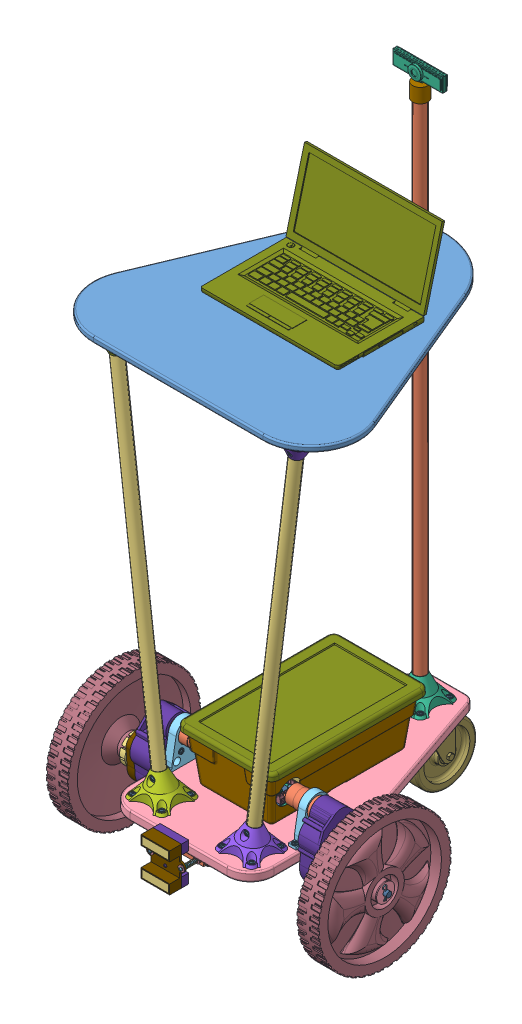
SolidWorks assembly Layla, configuration Default. Lengths in mm.
Overall size (589.28 1385.2 660.47).
388 component instances, 98 part files, 227 mates.
Components (placement in the parent):
- Layla_Top-1: Layla_Top [Default] at (-0.0562 830.9031 1403.6246) x (1 0 0.000267) z (-0.000267 0 1) size (558.8 12.7 558.8)
- Conduit_Back-1: Conduit_Back [Default] at (0.0274 577.85 997.2192) x (0.999959 0 0.009056) z (0 -1 0) size (24.13 24.13 1117.6)
- Conduit_Front-1: Conduit_Front [Default] at (144.1046 424.9766 1445.553) x (-0.000009 0 1) z (-0.121869 -0.992546 -0.000001) size (24.13 24.13 812.8)
- Conduit_Front-2: Conduit_Front [Default] at (-144.1046 424.9766 1445.553) x (0.000009 0 1) z (0.121869 -0.992546 -0.000001) size (24.13 24.13 812.8)
- Layla_Bottom-1: Layla_Bottom [Default] at (0.0001 0 1480.0562) x (1 0 0.000005) z (-0.000005 0 1) size (301.62 19.05 565.15)
- motor_bracket-1: motor_bracket [Default] at (128.32 -6.1562 1357.0318) x (0 1 0) z (1 0 0.000005) size (80.83 90 16)
- motor_bracket-2: motor_bracket [Default] at (-128.32 -6.1562 1357.0318) x (0 1 0) z (-1 0 0.000005) size (80.83 90 16)
- frame_bracket_volcano_back-1: frame_bracket_volcano_back [Default] at (0.0274 830.9031 997.2192) x (-0.00113 0 -0.999999) z (0 -1 0) size (90.91 90.9 52.13)
- frame_bracket_volcano_back-2: frame_bracket_volcano_back [Default] at (-0.0308 19.05 997.3051) x (-0.001001 0 -0.999999) z (0 1 0) size (90.91 90.9 52.13)
- frame_bracket_volcano_right-1: frame_bracket_volcano_right [Default] at (-94.2631 19.05 1445.5525) x (0.000009 0 1) z (0 1 0) size (90.91 90.9 53.32)
- frame_bracket_volcano_left-1: frame_bracket_volcano_left [Default] at (94.2631 19.05 1445.5525) x (-0.000009 0 1) z (0 -1 0) size (90.91 90.9 53.32)
- frame_bracket_volcano_right-2: frame_bracket_volcano_right [Default] at (-193.9461 830.9031 1445.5534) x (0.000009 0 1) z (0 -1 0) size (90.91 90.9 53.32)
- frame_bracket_volcano_left-2: frame_bracket_volcano_left [Default] at (193.9461 830.9031 1445.5534) x (-0.000009 0 1) z (0 1 0) size (90.91 90.9 53.32)
- Camera_Bracket-1: Camera_Bracket [Default] at (0.0274 1112.52 997.2192) x (0.105259 0 -0.994445) z (0.994445 0 0.105259) size (31.75 29.97 31.75)
- Axle_7_16-2: Axle_7_16 [Default] at (0.0008 -8.865 1357.1611) x (0.000005 -0.039071 -0.999236) z (1 0 0.000005) size (11.11 11.11 589.28)
- axle_bracket_7_16-1: axle_bracket_7_16 [Default] at (82.3318 -8.885 1357.1616) x (-0.000005 0 1) z (1 0 0.000005) size (44.81 15.79 16.5)
- axle_bracket_7_16-2: axle_bracket_7_16 [Default] at (-82.3303 -8.885 1357.1607) x (-0.000005 0 1) z (1 0 0.000005) size (44.81 15.79 16.5)
- Caster Part-1: Caster Part [Default] at (176.8474 -193.4184 944.9392) x (-1 0 -0.000005) z (0.000005 0 -1) size (73 156.46 148.87)
- 11in_Mower_Wheel-5: 11in_Mower_Wheel [Default] at (285.3317 -8.865 1357.1626) x (-0.000004 0.731602 0.681732) z (-1 0 -0.000005) size (279.4 279.4 57.46)
- 11in_Mower_Wheel-6: 11in_Mower_Wheel [Default] at (-285.3301 -8.865 1357.1596) x (-0.000005 0.394974 0.918692) z (1 0 0.000005) size (279.4 279.4 57.46)
- Screw_8_(0.75'')-1: Screw_8_(0.75'') [Default] at (-22.2101 9.652 1035.0706) x (-1 0 0) z (0 0 1) size (10.85 21.85 10.85)
- Screw_8_(0.75'')-2: Screw_8_(0.75'') [Default] at (22.2149 9.652 1035.0709) x (-1 0 0) z (0 0 1) size (10.85 21.85 10.85)
- Screw_8_(0.75'')-3: Screw_8_(0.75'') [Default] at (22.2153 9.652 958.9459) x (-1 0 0) z (0 0 1) size (10.85 21.85 10.85)
- Screw_8_(0.75'')-4: Screw_8_(0.75'') [Default] at (-22.2097 9.652 958.9456) x (-1 0 0) z (0 0 1) size (10.85 21.85 10.85)
- Screw_8_(0.75'')-5: Screw_8_(0.75'') [Default] at (82.3319 7.5213 1341.0054) x (-1 0 0) z (0 0 1) size (10.85 21.85 10.85)
- Screw_8_(0.75'')-7: Screw_8_(0.75'') [Default] at (-82.3303 7.5213 1373.3169) x (-1 0 0) z (0 0 1) size (10.85 21.85 10.85)
- Screw_8_(0.75'')-9: Screw_8_(0.75'') [Default] at (124.3148 10.35 1475.6049) x (-1 0 0) z (0 0 -1) size (10.85 21.85 10.85)
- Screw_8_(0.75'')-10: Screw_8_(0.75'') [Default] at (124.3154 10.35 1415.5008) x (-1 0 0) z (0 0 -1) size (10.85 21.85 10.85)
- Screw_8_(0.75'')-11: Screw_8_(0.75'') [Default] at (64.2113 10.35 1415.5002) x (-1 0 0) z (0 0 -1) size (10.85 21.85 10.85)
- Screw_8_(0.75'')-12: Screw_8_(0.75'') [Default] at (64.2107 10.35 1475.6043) x (-1 0 0) z (0 0 -1) size (10.85 21.85 10.85)
- Screw_8_(0.75'')-13: Screw_8_(0.75'') [Default] at (-64.2107 10.35 1475.6043) x (-1 0 0) z (0 0 -1) size (10.85 21.85 10.85)
- Screw_8_(0.75'')-14: Screw_8_(0.75'') [Default] at (-124.3148 10.35 1475.6049) x (-1 0 0) z (0 0 -1) size (10.85 21.85 10.85)
- Screw_8_(0.75'')-15: Screw_8_(0.75'') [Default] at (-124.3154 10.35 1415.5008) x (-1 0 0) z (0 0 -1) size (10.85 21.85 10.85)
- Screw_8_(0.75'')-17: Screw_8_(0.75'') [Default] at (-64.2113 10.35 1415.5002) x (-1 0 0) z (0 0 -1) size (10.85 21.85 10.85)
- Screw_8_(0.75'')-18: Screw_8_(0.75'') [Default] at (-136.3198 11.314 1395.7818) x (-1 0 0) z (0 0 -1) size (10.85 21.85 10.85)
- Screw_8_(0.75'')-19: Screw_8_(0.75'') [Default] at (-136.3202 11.314 1318.2818) x (-1 0 0) z (0 0 -1) size (10.85 21.85 10.85)
- Screw_8_(0.75'')-20: Screw_8_(0.75'') [Default] at (136.3198 11.314 1395.7818) x (-1 0 0) z (0 0 -1) size (10.85 21.85 10.85)
- Screw_8_(0.75'')-21: Screw_8_(0.75'') [Default] at (136.3202 11.314 1318.2818) x (-1 0 0) z (0 0 -1) size (10.85 21.85 10.85)
- Screw_8_(0.75'')-22: Screw_8_(0.75'') [Default] at (30.0513 10.35 1027.3271) x (-1 0 0) z (0 0 -1) size (10.85 21.85 10.85)
- Screw_8_(0.75'')-23: Screw_8_(0.75'') [Default] at (29.9912 10.35 967.223) x (-1 0 0) z (0 0 -1) size (10.85 21.85 10.85)
- Screw_8_(0.75'')-24: Screw_8_(0.75'') [Default] at (-30.1129 10.35 967.2832) x (-1 0 0) z (0 0 -1) size (10.85 21.85 10.85)
- Screw_8_(0.75'')-25: Screw_8_(0.75'') [Default] at (-30.0527 10.35 1027.3872) x (-1 0 0) z (0 0 -1) size (10.85 21.85 10.85)
- Screw_8_(0.75'')-28: Screw_8_(0.75'') [Default] at (-0.0319 56.55 996.1551) x (0 1 0) z (-0.999999 0 0.001001) size (10.85 21.85 10.85)
- Screw_8_(0.75'')-29: Screw_8_(0.75'') [Default] at (98.8331 56.2705 1446.7026) x (0 1 0) z (1 0 0.000009) size (10.85 21.85 10.85)
- Screw_8_(0.75'')-30: Screw_8_(0.75'') [Default] at (-98.8331 56.2705 1446.7026) x (0 1 0) z (1 0 -0.000009) size (10.85 21.85 10.85)
- Screw_8_(0.75'')-32: Screw_8_(0.75'') [Default] at (-189.376 793.6826 1446.7034) x (0 -1 0) z (-1 0 0.000009) size (10.85 21.85 10.85)
- Screw_8_(0.75'')-33: Screw_8_(0.75'') [Default] at (189.376 793.6826 1446.7034) x (0 1 0) z (1 0 0.000009) size (10.85 21.85 10.85)
- Screw_8_(0.75'')-34: Screw_8_(0.75'') [Default] at (0.0261 793.4031 996.0692) x (0 1 0) z (-0.999999 0 0.00113) size (10.85 21.85 10.85)
- Screw_8_(0.75'')-36: Screw_8_(0.75'') [Default] at (82.3317 7.5213 1373.3178) x (-1 0 0) z (0 0 1) size (10.85 21.85 10.85)
- Screw_8_(0.75'')-37: Screw_8_(0.75'') [Default] at (-82.3302 7.5213 1341.0045) x (-1 0 0) z (0 0 1) size (10.85 21.85 10.85)
- Screw_8_(0.75'')-38: Screw_8_(0.75'') [Default] at (-141.0199 47.7688 1371.1468) x (0.000005 0 1) z (0 1 0) size (10.85 21.85 10.85)
- Screw_8_(0.75'')-39: Screw_8_(0.75'') [Default] at (141.0201 47.7688 1342.9169) x (0.000005 0 -1) z (0 1 0) size (10.85 21.85 10.85)
- Screw_8_(0.5'')-1: Screw_8_(0.5'') [Default] at (223.9979 833.2531 1475.6057) x (-1 0 -0.000267) z (-0.000267 0 1) size (10.85 15.5 10.85)
- Screw_8_(0.5'')-2: Screw_8_(0.5'') [Default] at (163.8938 833.2531 1475.6052) x (-1 0 -0.000267) z (-0.000267 0 1) size (10.85 15.5 10.85)
- Screw_8_(0.5'')-3: Screw_8_(0.5'') [Default] at (163.8943 833.2531 1415.5011) x (-1 0 -0.000267) z (-0.000267 0 1) size (10.85 15.5 10.85)
- Screw_8_(0.5'')-4: Screw_8_(0.5'') [Default] at (223.9984 833.2531 1415.5017) x (-1 0 -0.000267) z (-0.000267 0 1) size (10.85 15.5 10.85)
- Screw_8_(0.5'')-6: Screw_8_(0.5'') [Default] at (-163.8938 833.2531 1475.6052) x (-1 0 -0.000267) z (-0.000267 0 1) size (10.85 15.5 10.85)
- Screw_8_(0.5'')-7: Screw_8_(0.5'') [Default] at (-223.9979 833.2531 1475.6057) x (-1 0 -0.000267) z (-0.000267 0 1) size (10.85 15.5 10.85)
- Screw_8_(0.5'')-8: Screw_8_(0.5'') [Default] at (-223.9984 833.2531 1415.5017) x (-1 0 -0.000267) z (-0.000267 0 1) size (10.85 15.5 10.85)
- Screw_8_(0.5'')-9: Screw_8_(0.5'') [Default] at (-163.8943 833.2531 1415.5011) x (-1 0 -0.000267) z (-0.000267 0 1) size (10.85 15.5 10.85)
- Screw_8_(0.5'')-10: Screw_8_(0.5'') [Default] at (30.1134 833.2531 1027.2373) x (-1 0 -0.000267) z (-0.000267 0 1) size (10.85 15.5 10.85)
- Screw_8_(0.5'')-11: Screw_8_(0.5'') [Default] at (-29.9907 833.2531 1027.3052) x (-1 0 -0.000267) z (-0.000267 0 1) size (10.85 15.5 10.85)
- Screw_8_(0.5'')-12: Screw_8_(0.5'') [Default] at (-30.0586 833.2531 967.2011) x (-1 0 -0.000267) z (-0.000267 0 1) size (10.85 15.5 10.85)
- Screw_8_(0.5'')-13: Screw_8_(0.5'') [Default] at (30.0455 833.2531 967.1332) x (-1 0 -0.000267) z (-0.000267 0 1) size (10.85 15.5 10.85)
- Laptop-2: Laptop [Default] at (-144.399 841.3074 1314.5854) size (290.36 165.51 224.16)
- Peg_Perego_Gearbox-1: Peg_Perego_Gearbox [Default] at (178.15 45.4709 1342.5236) x (0.000001 0.992561 -0.121745) z (-0.000005 0.121745 0.992561) size (150.54 143.03 103.18)
  - Peg_Perego_Gearbox_Bottom-1: Peg_Perego_Gearbox_Bottom [Default] at (-27.6979 -16.6053 10.3143) size (150.54 43.95 103.18)
  - Peg_Perego_Gearbox_Top-1: Peg_Perego_Gearbox_Top [Default] at (-40.5901 -16.6053 7.9144) x (-1 0 0) z (0 0 1) size (114.07 19.3 83.82)
  - Peg_Perego_Gearbox_Big_Gear-1: Peg_Perego_Gearbox_Big_Gear [Default] at (-55.7139 -16.6053 7.9144) x (-1 0 0) z (0 0 1) size (53.24 35.08 53.24)
  - Peg_Perego_Gearbox_Motor-1: Peg_Perego_Gearbox_Motor [Default] at (26.8065 84.3597 18.0362) x (0 0 1) z (1 0 0) size (37.46 84.84 37.46)
- Peg_Perego_Gearbox-8: Peg_Perego_Gearbox [Default] at (-178.1485 45.5433 1371.527) x (-0.000001 0.993157 0.116786) z (0.000005 0.116786 -0.993157) size (150.54 143.03 103.18)
  - Peg_Perego_Gearbox_Bottom-1: Peg_Perego_Gearbox_Bottom [Default] at (-27.6979 -16.6053 10.3143) size (150.54 43.95 103.18)
  - Peg_Perego_Gearbox_Top-1: Peg_Perego_Gearbox_Top [Default] at (-40.5901 -16.6053 7.9144) x (-1 0 0) z (0 0 1) size (114.07 19.3 83.82)
  - Peg_Perego_Gearbox_Big_Gear-1: Peg_Perego_Gearbox_Big_Gear [Default] at (-55.7139 -16.6053 7.9144) x (-1 0 0) z (0 0 1) size (53.24 35.08 53.24)
  - Peg_Perego_Gearbox_Motor-1: Peg_Perego_Gearbox_Motor [Default] at (26.8065 84.3597 18.0362) x (0 0 1) z (1 0 0) size (37.46 84.84 37.46)
- 11in_barbie_mower-1: 11in_barbie_mower [Default] at (241.7707 -8.865 1357.1624) x (0.000005 -0.121745 -0.992561) z (0.000001 0.992561 -0.121745) size (59.94 28.01 59.94)
- 11in_barbie_mower-3: 11in_barbie_mower [Default] at (-241.7691 -8.865 1357.1599) x (0.000001 -0.993157 -0.116786) z (-0.000005 -0.116786 0.993157) size (59.94 28.01 59.94)
- Washer_7_16-1: Washer_7_16 [Default] at (-287.3621 -8.865 1357.1596) x (-0.000004 0.592783 0.805362) z (1 0 0.000005) size (38.1 38.1 2.03)
- Washer_7_16-2: Washer_7_16 [Default] at (285.3317 -8.865 1357.1626) x (-0.000003 0.8256 0.564257) z (1 0 0.000005) size (38.1 38.1 2.03)
- Hair Pin Cotter Pin-1: Hair Pin Cotter Pin [Default] at (288.7988 -22.9437 1357.7131) x (0 0.999236 -0.039071) z (-0.000005 0.039071 0.999236) size (30.72 1.5 9.05)
- Hair Pin Cotter Pin-2: Hair Pin Cotter Pin [Default] at (-288.7972 -22.6511 1357.6986) x (0 0.999236 -0.039071) z (-0.000005 0.039071 0.999236) size (30.72 1.5 9.05)
- Genius_Webcam-1: Genius_Webcam [Default] at (0.0274 1163.8661 993.1679) size (105.03 41.22 29.03)
- Counterweight_Ingot-1: Counterweight_Ingot [Default] at (0.0022 0 1072.91) x (1 0 0.000005) z (0.000005 0 -1) size (106.83 31.75 49.05)
- Counterweight_Ingot_Screw-1: Counterweight_Ingot_Screw [Default] at (-28.5728 -32.25 1072.9098) x (-1 0 0) z (0 0 1) size (8 45 8)
- Counterweight_Ingot_Screw-2: Counterweight_Ingot_Screw [Default] at (28.5772 -32.25 1072.9101) x (-1 0 0) z (0 0 1) size (8 45 8)
- electronics_box-2: electronics_box [Default] at (6.4079 61.0311 1230.8661) x (-1 0 -0.000005) z (0.000005 0 -1) size (200.66 116.21 330.83)
  - sterilite_box-1: sterilite_box [Default] at (6.4065 -41.9824 -170.8478) size (195.22 114.3 325.39)
  - electronics_tray-1: electronics_tray [Default] at (67.0566 -75.9526 -72.8113) x (0 0 1) z (-1 0 0) size (203.2 36.13 152.4)
    - ibt2_assembly-1: ibt2_assembly [Default] at (25.1982 40.7289 22.1019) size (49.66 21.28 49.78)
      - IBT2_pcb-1: IBT2_pcb [Default] at (-57.2691 7.2367 24.7687) size (49.66 1.57 49.4)
      - header_male_2x4-1: header_male_2x4 [Default] at (4.8115 23.0826 24.5335) x (1 0 0) z (0 -1 0) size (10.16 5.08 10.92)
        - header_pin_base_2x4-1: header_pin_base_2x4 [Default] at (-49.9521 21.6346 11.7311) size (10.16 5.08 2.54)
        - header_pin-1: header_pin [Default] at (-56.3021 22.9046 6.0161) size (0.64 0.64 10.92)
        - header_pin-2: header_pin [Default] at (-56.3021 20.3646 6.0161) size (0.64 0.64 10.92)
        - header_pin-3: header_pin [Default] at (-53.7621 22.9046 6.0161) size (0.64 0.64 10.92)
        - header_pin-4: header_pin [Default] at (-53.7621 20.3646 6.0161) size (0.64 0.64 10.92)
        - header_pin-5: header_pin [Default] at (-51.2221 22.9046 6.0161) size (0.64 0.64 10.92)
        - header_pin-6: header_pin [Default] at (-51.2221 20.3646 6.0161) size (0.64 0.64 10.92)
        - header_pin-7: header_pin [Default] at (-48.6821 22.9046 6.0161) size (0.64 0.64 10.92)
        - header_pin-8: header_pin [Default] at (-48.6821 20.3646 6.0161) size (0.64 0.64 10.92)
      - AMP_screw-terminal_2POS_large-1: AMP_screw-terminal_2POS_large [Default] at (-57.2056 17.0115 0.4662) x (-1 0 0) z (0 0 -1) size (10.66 17 9)
      - AMP_screw-terminal_2POS_large-2: AMP_screw-terminal_2POS_large [Default] at (-47.0456 17.0115 0.4662) x (-1 0 0) z (0 0 -1) size (10.66 17 9)
      - cap_5mm_pitch-1: cap_5mm_pitch [Default] at (-68.3924 8.8115 4.7662) size (10.16 19.69 10.16)
      - d2pak-1: d2pak [Default] at (-63.2409 8.7779 25.6248) x (1 0 0) z (0 0.999978 0.006671) size (9.87 15.09 4.26)
      - d2pak-2: d2pak [Default] at (-52.336 8.7779 25.6248) x (1 0 0) z (0 0.999978 0.006671) size (9.87 15.09 4.26)
      - SOIC20 wide-1: SOIC20 wide [Default] at (-39.9304 8.5615 36.0347) x (1 0 0) z (0 1 0) size (13 10.17 2.01)
      - cap_0805-1: cap_0805 [Default] at (-38.0286 9.3449 27.3468) x (1 0 0) z (0 -1 0) size (2.03 1.32 0.56)
      - resistor_0805-1: resistor_0805 [Default] at (-48.3156 9.3449 41.6216) x (0 0 -1) z (0 -1 0) size (2.03 1.32 0.56)
      - resistor_0805-2: resistor_0805 [Default] at (-50.4517 9.3449 41.6216) x (0 0 -1) z (0 -1 0) size (2.03 1.32 0.56)
      - resistor_0805-3: resistor_0805 [Default] at (-52.5879 9.3449 41.6216) x (0 0 -1) z (0 -1 0) size (2.03 1.32 0.56)
      - resistor_0805-4: resistor_0805 [Default] at (-54.724 9.3449 41.6216) x (0 0 -1) z (0 -1 0) size (2.03 1.32 0.56)
      - resistor_0805-5: resistor_0805 [Default] at (-56.8602 9.3449 41.6216) x (0 0 -1) z (0 -1 0) size (2.03 1.32 0.56)
      - resistor_0805-6: resistor_0805 [Default] at (-58.9963 9.3449 41.6216) x (0 0 -1) z (0 -1 0) size (2.03 1.32 0.56)
      - resistor_0805-7: resistor_0805 [Default] at (-61.1324 9.3449 41.6216) x (0 0 -1) z (0 -1 0) size (2.03 1.32 0.56)
      - resistor_0805-8: resistor_0805 [Default] at (-63.2686 9.3449 41.6216) x (0 0 -1) z (0 -1 0) size (2.03 1.32 0.56)
    - ibt2_assembly-2: ibt2_assembly [Default] at (-89.34 40.7289 121.0422) x (-1 0 0) z (0 0 -1) size (49.66 21.28 49.78)
      - IBT2_pcb-1: IBT2_pcb [Default] at (-57.2691 7.2367 24.7687) size (49.66 1.57 49.4)
      - header_male_2x4-1: header_male_2x4 [Default] at (4.8115 23.0826 24.5335) x (1 0 0) z (0 -1 0) size (10.16 5.08 10.92)
        - header_pin_base_2x4-1: header_pin_base_2x4 [Default] at (-49.9521 21.6346 11.7311) size (10.16 5.08 2.54)
        - header_pin-1: header_pin [Default] at (-56.3021 22.9046 6.0161) size (0.64 0.64 10.92)
        - header_pin-2: header_pin [Default] at (-56.3021 20.3646 6.0161) size (0.64 0.64 10.92)
        - header_pin-3: header_pin [Default] at (-53.7621 22.9046 6.0161) size (0.64 0.64 10.92)
        - header_pin-4: header_pin [Default] at (-53.7621 20.3646 6.0161) size (0.64 0.64 10.92)
        - header_pin-5: header_pin [Default] at (-51.2221 22.9046 6.0161) size (0.64 0.64 10.92)
        - header_pin-6: header_pin [Default] at (-51.2221 20.3646 6.0161) size (0.64 0.64 10.92)
        - header_pin-7: header_pin [Default] at (-48.6821 22.9046 6.0161) size (0.64 0.64 10.92)
        - header_pin-8: header_pin [Default] at (-48.6821 20.3646 6.0161) size (0.64 0.64 10.92)
      - AMP_screw-terminal_2POS_large-1: AMP_screw-terminal_2POS_large [Default] at (-57.2056 17.0115 0.4662) x (-1 0 0) z (0 0 -1) size (10.66 17 9)
      - AMP_screw-terminal_2POS_large-2: AMP_screw-terminal_2POS_large [Default] at (-47.0456 17.0115 0.4662) x (-1 0 0) z (0 0 -1) size (10.66 17 9)
      - cap_5mm_pitch-1: cap_5mm_pitch [Default] at (-68.3924 8.8115 4.7662) size (10.16 19.69 10.16)
      - d2pak-1: d2pak [Default] at (-63.2409 8.7779 25.6248) x (1 0 0) z (0 0.999978 0.006671) size (9.87 15.09 4.26)
      - d2pak-2: d2pak [Default] at (-52.336 8.7779 25.6248) x (1 0 0) z (0 0.999978 0.006671) size (9.87 15.09 4.26)
      - SOIC20 wide-1: SOIC20 wide [Default] at (-39.9304 8.5615 36.0347) x (1 0 0) z (0 1 0) size (13 10.17 2.01)
      - cap_0805-1: cap_0805 [Default] at (-38.0286 9.3449 27.3468) x (1 0 0) z (0 -1 0) size (2.03 1.32 0.56)
      - resistor_0805-1: resistor_0805 [Default] at (-48.3156 9.3449 41.6216) x (0 0 -1) z (0 -1 0) size (2.03 1.32 0.56)
      - resistor_0805-2: resistor_0805 [Default] at (-50.4517 9.3449 41.6216) x (0 0 -1) z (0 -1 0) size (2.03 1.32 0.56)
      - resistor_0805-3: resistor_0805 [Default] at (-52.5879 9.3449 41.6216) x (0 0 -1) z (0 -1 0) size (2.03 1.32 0.56)
      - resistor_0805-4: resistor_0805 [Default] at (-54.724 9.3449 41.6216) x (0 0 -1) z (0 -1 0) size (2.03 1.32 0.56)
      - resistor_0805-5: resistor_0805 [Default] at (-56.8602 9.3449 41.6216) x (0 0 -1) z (0 -1 0) size (2.03 1.32 0.56)
      - resistor_0805-6: resistor_0805 [Default] at (-58.9963 9.3449 41.6216) x (0 0 -1) z (0 -1 0) size (2.03 1.32 0.56)
      - resistor_0805-7: resistor_0805 [Default] at (-61.1324 9.3449 41.6216) x (0 0 -1) z (0 -1 0) size (2.03 1.32 0.56)
      - resistor_0805-8: resistor_0805 [Default] at (-63.2686 9.3449 41.6216) x (0 0 -1) z (0 -1 0) size (2.03 1.32 0.56)
    - Arduino_mega-1: Arduino_mega [Default] at (5.4045 37.4555 130.5264) x (0 0 1) z (0 1 0) size (107.7 53.34 12.38)
      - Arduino_mega-1: Arduino_mega [Default] at (-98.4513 -6.297 10.51) size (101.6 53.34 1.59)
      - USB-jack-1: USB-jack [Default] at (-104.5473 25.6308 12.0975) size (16.46 12.14 10.79)
      - DC-jack-1: DC-jack [Default] at (-99.9245 -2.5632 12.0975) x (0 1 0) z (0 0 -1) size (8.79 13.59 10.72)
      - header_8-pin-1: header_8-pin [Default] at (-53.7727 -5.0778 12.0975) size (20.32 2.54 8.56)
      - header_8-pin-2: header_8-pin [Default] at (-30.6587 -5.0778 12.0975) size (20.32 2.54 8.56)
      - header_8-pin-3: header_8-pin [Default] at (-8.0781 -5.0778 12.0975) size (20.32 2.54 8.56)
      - header_8-pin-4: header_8-pin [Default] at (-35.7895 43.0044 12.0975) size (20.32 2.54 8.56)
      - header_8-pin-5: header_8-pin [Default] at (-13.1835 43.0044 12.0975) size (20.32 2.54 8.56)
      - header_10-pin-1: header_10-pin [Default] at (-58.0145 43.0044 12.0975) size (25.4 2.54 8.56)
      - header_36-pin-1: header_36-pin [Default] at (-0.5343 43.0298 12.0975) x (0 1 0) z (0 0 1) size (45.72 5.08 8.56)
    - arduino uno-1: arduino uno [Default] at (57.5276 49.6156 28.9001) x (-1 0 0) z (0 0 -1) size (53.34 15.25 74.97)
      - unoboard blue-1: unoboard blue [Default] at origin size (53.34 1.65 68.58)
      - 47uf CAP Dcase-1: 47uf CAP Dcase [Default] at (-9.4141 0 -18.4991) x (0 0 -1) z (1 0 0) size (6.6 5.81 8)
      - USB type b-1: USB type b [Default] at (-38.02 0.43 6.35) size (13.72 15.2 16.54)
        - USB SHELL-1: USB SHELL [Default] at origin size (13.72 15.2 16.54)
        - USB core-1: USB core [Default] at origin size (11.3 10.68 15.75)
        - usb top contact-1: usb top contact [Default] at (1.25 6.09 -0.38) size (1 9.67 13.76)
        - usb btm contact-1: usb btm contact [Default] at (1.25 4.41 -0.38) size (1 6.84 11.76)
        - usb btm contact-2: usb btm contact [Default] at (-1.25 4.41 -0.38) size (1 6.84 11.76)
        - usb top contact-2: usb top contact [Default] at (-1.25 6.09 -0.38) size (1 9.67 13.76)
      - power jack-1: power jack [Default] at (-7.675 0 1.905) size (11.2 15.2 15.9)
      - 47uf CAP Dcase-2: 47uf CAP Dcase [Default] at (-9.4141 0 -25.7132) x (0 0 -1) z (1 0 0) size (6.6 5.81 8)
      - crystal-1: crystal [Default] at (-26.162 0 -18.923) x (1 0 0) z (0 0 -1) size (4 5 11)
      - 2pin_header__02-1: 2pin_header__02 [Default] at (-46.23 0 -15.75) size (5 11.75 2.54)
      - nano - reg-1: nano - reg [Default] at (-17.399 0 -7.747) size (6.5 1.69 8.3)
      - led-1: led [Default] at (-34.29 0 -27.94) x (0 0 1) z (-1 0 0) size (4 0.86 1.35)
      - 2pin_header__02-2: 2pin_header__02 [Default] at (-30.43 0 -64.91) x (0 0 1) z (-1 0 0) size (5 11.75 2.54)
      - dip28-1: dip28 [Default] at (-16.383 1.5 -46.355) x (0 0 -1) z (1 0 0) size (35.48 7.37 10.1)
        - dip28-1: dip28 [Default] at origin size (35.48 2.8 10.1)
        - dip socket pin-1: dip socket pin [Default] at (16.51 2.8 -3.81) size (1.7 7.37 1.7)
        - dip socket pin-2: dip socket pin [Default] at (16.51 2.8 3.81) size (1.7 7.37 1.7)
        - dip socket pin-3: dip socket pin [Default] at (13.97 2.8 -3.81) size (1.7 7.37 1.7)
        - dip socket pin-4: dip socket pin [Default] at (13.97 2.8 3.81) size (1.7 7.37 1.7)
        - dip socket pin-5: dip socket pin [Default] at (11.43 2.8 -3.81) size (1.7 7.37 1.7)
        - dip socket pin-6: dip socket pin [Default] at (11.43 2.8 3.81) size (1.7 7.37 1.7)
        - dip socket pin-7: dip socket pin [Default] at (8.89 2.8 -3.81) size (1.7 7.37 1.7)
        - dip socket pin-8: dip socket pin [Default] at (8.89 2.8 3.81) size (1.7 7.37 1.7)
        - dip socket pin-9: dip socket pin [Default] at (6.35 2.8 -3.81) size (1.7 7.37 1.7)
        - dip socket pin-10: dip socket pin [Default] at (6.35 2.8 3.81) size (1.7 7.37 1.7)
        - dip socket pin-11: dip socket pin [Default] at (3.81 2.8 -3.81) size (1.7 7.37 1.7)
        - dip socket pin-12: dip socket pin [Default] at (3.81 2.8 3.81) size (1.7 7.37 1.7)
        - dip socket pin-13: dip socket pin [Default] at (1.27 2.8 -3.81) size (1.7 7.37 1.7)
        - dip socket pin-14: dip socket pin [Default] at (1.27 2.8 3.81) size (1.7 7.37 1.7)
        - dip socket pin-15: dip socket pin [Default] at (-1.27 2.8 -3.81) size (1.7 7.37 1.7)
        - dip socket pin-16: dip socket pin [Default] at (-1.27 2.8 3.81) size (1.7 7.37 1.7)
        - dip socket pin-17: dip socket pin [Default] at (-3.81 2.8 -3.81) size (1.7 7.37 1.7)
        - dip socket pin-18: dip socket pin [Default] at (-3.81 2.8 3.81) size (1.7 7.37 1.7)
        - dip socket pin-19: dip socket pin [Default] at (-6.35 2.8 -3.81) size (1.7 7.37 1.7)
        - dip socket pin-20: dip socket pin [Default] at (-6.35 2.8 3.81) size (1.7 7.37 1.7)
        - dip socket pin-21: dip socket pin [Default] at (-8.89 2.8 -3.81) size (1.7 7.37 1.7)
        - dip socket pin-22: dip socket pin [Default] at (-8.89 2.8 3.81) size (1.7 7.37 1.7)
        - dip socket pin-23: dip socket pin [Default] at (-11.43 2.8 -3.81) size (1.7 7.37 1.7)
        - dip socket pin-24: dip socket pin [Default] at (-11.43 2.8 3.81) size (1.7 7.37 1.7)
        - dip socket pin-25: dip socket pin [Default] at (-13.97 2.8 -3.81) size (1.7 7.37 1.7)
        - dip socket pin-26: dip socket pin [Default] at (-13.97 2.8 3.81) size (1.7 7.37 1.7)
        - dip socket pin-27: dip socket pin [Default] at (-16.51 2.8 -3.81) size (1.7 7.37 1.7)
        - dip socket pin-28: dip socket pin [Default] at (-16.51 2.8 3.81) size (1.7 7.37 1.7)
      - 2pin_header__02-3: 2pin_header__02 [Default] at (-27.89 0 -64.91) x (0 0 1) z (-1 0 0) size (5 11.75 2.54)
      - 2pin_header__02-4: 2pin_header__02 [Default] at (-25.35 0 -64.91) x (0 0 1) z (-1 0 0) size (5 11.75 2.54)
      - 2pin_header__02-5: 2pin_header__02 [Default] at (-46.23 0 -18.29) size (5 11.75 2.54)
      - 2pin_header__02-6: 2pin_header__02 [Default] at (-46.23 0 -20.83) size (5 11.75 2.54)
      - atmega16u2-1: atmega16u2 [Default] at (-34.671 0.06 -20) x (1 0 0) z (0 0 -1) size (5.5 1.01 5.5)
      - led-2: led [Default] at (-36.83 0 -27.94) x (0 0 1) z (-1 0 0) size (4 0.86 1.35)
      - led-3: led [Default] at (-42.037 0 -27.94) x (0 0 1) z (-1 0 0) size (4 0.86 1.35)
      - led-4: led [Default] at (-36.576 0 -58.42) x (0 0 1) z (-1 0 0) size (4 0.86 1.35)
      - 8 PORT HEADER-3: 8 PORT HEADER [Default] at (-50.8 0 -45.72) x (0 0 -1) z (1 0 0) size (20.32 10.51 2.41)
      - 8 PORT HEADER-4: 8 PORT HEADER [Default] at (-2.54 0 -27.94) x (0 0 -1) z (1 0 0) size (20.32 10.51 2.41)
      - 6 PORT HEADER-3: 6 PORT HEADER [Default] at (-2.54 0 -50.8) x (0 0 -1) z (1 0 0) size (15.24 10.51 2.41)
      - 10 PORT HEADER-1: 10 PORT HEADER [Default] at (-50.8 0 -18.796) x (0 0 -1) z (1 0 0) size (25.4 10.51 2.41)
      - ATMEL328P-1: ATMEL328P [Default] at (-16.383 4.3 -46.355) x (0 0 -1) z (1 0 0) size (35 7.27 7.87)
      - 102 RESISTOR PACK-1: 102 RESISTOR PACK [Default] at (-33.782 0 -58.42) size (3.2 0.46 3)
      - 102 RESISTOR PACK-2: 102 RESISTOR PACK [Default] at (-39.37 0 -27.94) size (3.2 0.46 3)
      - 103 RESISTOR PACK-3: 103 RESISTOR PACK [Default] at (-23.876 0 -27.94) size (3.2 0.46 3)
      - 220 RESISTOR PACK-1: 220 RESISTOR PACK [Default] at (-36.83 0 -12.827) size (3.2 0.46 3)
      - 16mhz crystal - measured-1: 16mhz crystal - measured [Default] at (-24.892 0 -41.275) x (0 0 -1) z (1 0 0) size (3.4 0.8 2)
      - PADS001-1: PADS001 [Default] at (-39.878 0.1 -18.288) x (-1 0 0) z (0 0 1) size (4.54 0.1 4.54)
      - 603 cap on pad-1: 603 cap on pad [Default] at (-44.45 0 -27.94) x (0 0 -1) z (1 0 0) size (2.76 0.9 1.12)
      - ssot3-1: ssot3 [Default] at (-26.5 0 -8.128) x (-1 0 0) z (0 0 -1) size (3 1.13 3.09)
      - mf-msmf050-2-1: mf-msmf050-2 [Default] at (-26.5 0 -4.064) size (5.77 1.02 3.72)
      - 603 cap on pad-2: 603 cap on pad [Default] at (-29.845 0 -27.94) x (0 0 -1) z (1 0 0) size (2.76 0.9 1.12)
      - 603 cap on pad-3: 603 cap on pad [Default] at (-31.496 0 -27.94) x (0 0 -1) z (1 0 0) size (2.76 0.9 1.12)
      - lmv358-1: lmv358 [Default] at (-15.24 0 -21.971) x (0 0 -1) z (1 0 0) size (3.7 1.4 2.9)
      - 603 cap on pad-4: 603 cap on pad [Default] at (-15.24 0 -18.415) size (2.76 0.9 1.12)
      - 603 cap on pad-5: 603 cap on pad [Default] at (-29.845 0 -12.065) x (0 0 1) z (-1 0 0) size (2.76 0.9 1.12)
      - 603 cap on pad-6: 603 cap on pad [Default] at (-29.591 0 -22.352) x (0 0 1) z (-1 0 0) size (2.76 0.9 1.12)
      - 603 cap on pad-7: 603 cap on pad [Default] at (-29.591 0 -16.002) x (0 0 1) z (-1 0 0) size (2.76 0.9 1.12)
      - 603 cap on pad-8: 603 cap on pad [Default] at (-41.91 0 -12.7) x (0 0 1) z (-1 0 0) size (2.76 0.9 1.12)
      - lp2985dgkr-1: lp2985dgkr [Default] at (-20.32 0 -19.05) x (0 0 -1) z (1 0 0) size (5.85 1.1 3)
      - cd1206 diode-1: cd1206 diode [Default] at (-27.94 0 -59.436) x (0 0 -1) z (1 0 0) size (2.07 0.96 5)
      - cd1206 diode-2: cd1206 diode [Default] at (-46.228 0 -13.081) x (0 0 1) z (-1 0 0) size (2.07 0.96 5)
      - 603 resistor-1: 603 resistor [Default] at (-29.591 0 -19.05) x (0 0 1) z (-1 0 0) size (2.36 0.61 1.03)
      - blm21-1: blm21 [Default] at (-45.085 0 -7.62) x (0 0 -1) z (1 0 0) size (2.76 0.95 1.32)
      - m7 diode-1: m7 diode [Default] at (-2.794 0 -21.59) x (0 0 -1) z (1 0 0) size (6.66 2.35 2.5)
      - MLC0603-1: MLC0603 [Default] at (-33.655 0 -12.827) x (0 0 -1) z (1 0 0) size (2.36 0.6 1.03)
      - MLC0603-2: MLC0603 [Default] at (-39.37 0 -12.827) x (0 0 -1) z (1 0 0) size (2.36 0.6 1.03)
      - RESET BUTTON-1: RESET BUTTON [Default] at (-49.403 0 -6.35) size (6.2 3.1 9.6)
        - RESET CORE-1: RESET CORE [Default] at (0 0.1 0) x (-1 0 0) z (0 0 -1) size (6.2 3.1 9.6)
        - RESET-1: RESET [Default] at (0 0.1 0) x (0 0 1) z (-1 0 0) size (7.3 2 6.2)
      - 603 cap on pad-9: 603 cap on pad [Default] at (-15.24 0 -25.625) size (2.76 0.9 1.12)
    - electronics_tray_tray-1: electronics_tray_tray [Default] at origin size (203.2 13.95 152.4)
    - m3x6mm_cap_screw-1: m3x6mm_cap_screw [92095A179] at (-11.9414 51.1904 27.3507) x (-0.837169 0 -0.546944) z (0 1 0) size (5.7 5.7 7.77)
    - bms_assembly-1: bms_assembly [Default] at (83.3041 41.8308 46.3558) x (0 0 -1) z (0 1 0) size (88.9 53.34 22.95)
      - bms_board-1: bms_board [Default] at (-80.72 -27.381 18.8348) size (88.9 53.34 1.57)
      - AMP_screw-terminal_2POS_large-1: AMP_screw-terminal_2POS_large [Default] at (-79.94 10.719 28.6096) x (0 -1 0) z (-1 0 0) size (10.66 17 9)
      - AMP_screw-terminal_2POS_large-2: AMP_screw-terminal_2POS_large [Default] at (-79.94 0.559 28.6096) x (0 -1 0) z (-1 0 0) size (10.66 17 9)
      - B4B-XH-Apart-1: B4B-XH-Apart [Default] at (-77.791 -14.995 20.4096) x (0 1 0) z (1 0 0) size (12.4 10.4 5.75)
      - header_male_1x10-1: header_male_1x10 [Default] at (49.0022 32.4877 36.1995) x (0 1 0) z (0 0 1) size (2.54 25.4 10.92)
        - header_pin-1: header_pin [Default] at (-57.3287 73.639 -25.2387) size (0.64 0.64 10.92)
        - header_pin_base_single-1: header_pin_base_single [Default] at (-58.5987 72.369 -19.9047) size (2.54 2.54 2.54)
        - header_pin_base_single-2: header_pin_base_single [Default] at (-58.5987 69.829 -19.9047) size (2.54 2.54 2.54)
        - header_pin_base_single-3: header_pin_base_single [Default] at (-58.5987 67.289 -19.9047) size (2.54 2.54 2.54)
        - header_pin_base_single-4: header_pin_base_single [Default] at (-58.5987 64.749 -19.9047) size (2.54 2.54 2.54)
        - header_pin_base_single-5: header_pin_base_single [Default] at (-58.5987 62.209 -19.9047) size (2.54 2.54 2.54)
        - header_pin_base_single-6: header_pin_base_single [Default] at (-58.5987 59.669 -19.9047) size (2.54 2.54 2.54)
        - header_pin-2: header_pin [Default] at (-57.3287 71.099 -25.2387) size (0.64 0.64 10.92)
        - header_pin-3: header_pin [Default] at (-57.3287 68.559 -25.2387) size (0.64 0.64 10.92)
        - header_pin-4: header_pin [Default] at (-57.3287 66.019 -25.2387) size (0.64 0.64 10.92)
        - header_pin-5: header_pin [Default] at (-57.3287 63.479 -25.2387) size (0.64 0.64 10.92)
        - header_pin-6: header_pin [Default] at (-57.3287 60.939 -25.2387) size (0.64 0.64 10.92)
        - header_pin-7: header_pin [Default] at (-57.3287 58.399 -25.2387) size (0.64 0.64 10.92)
        - header_pin-8: header_pin [Default] at (-57.3287 55.859 -25.2387) size (0.64 0.64 10.92)
        - header_pin_base_single-7: header_pin_base_single [Default] at (-58.5987 57.129 -19.9047) size (2.54 2.54 2.54)
        - header_pin_base_single-8: header_pin_base_single [Default] at (-58.5987 54.589 -19.9047) size (2.54 2.54 2.54)
        - header_pin_base_single-9: header_pin_base_single [Default] at (-58.5987 52.049 -19.9047) size (2.54 2.54 2.54)
        - header_pin_base_single-10: header_pin_base_single [Default] at (-58.5987 49.509 -19.9047) size (2.54 2.54 2.54)
        - header_pin-9: header_pin [Default] at (-57.3287 53.319 -25.2387) size (0.64 0.64 10.92)
        - header_pin-10: header_pin [Default] at (-57.3287 50.779 -25.2387) size (0.64 0.64 10.92)
      - header_male_1x8-1: header_male_1x8 [Default] at (-84.3058 -33.9097 36.1995) x (0 -1 0) z (0 0 1) size (2.54 20.32 10.92)
        - header_pin-1: header_pin [Default] at (-57.3287 73.639 -25.2387) size (0.64 0.64 10.92)
        - header_pin_base_single-1: header_pin_base_single [Default] at (-58.5987 72.369 -19.9047) size (2.54 2.54 2.54)
        - header_pin_base_single-2: header_pin_base_single [Default] at (-58.5987 69.829 -19.9047) size (2.54 2.54 2.54)
        - header_pin_base_single-3: header_pin_base_single [Default] at (-58.5987 67.289 -19.9047) size (2.54 2.54 2.54)
        - header_pin_base_single-4: header_pin_base_single [Default] at (-58.5987 64.749 -19.9047) size (2.54 2.54 2.54)
        - header_pin_base_single-5: header_pin_base_single [Default] at (-58.5987 62.209 -19.9047) size (2.54 2.54 2.54)
        - header_pin_base_single-6: header_pin_base_single [Default] at (-58.5987 59.669 -19.9047) size (2.54 2.54 2.54)
        - header_pin-2: header_pin [Default] at (-57.3287 71.099 -25.2387) size (0.64 0.64 10.92)
        - header_pin-3: header_pin [Default] at (-57.3287 68.559 -25.2387) size (0.64 0.64 10.92)
        - header_pin-4: header_pin [Default] at (-57.3287 66.019 -25.2387) size (0.64 0.64 10.92)
        - header_pin-5: header_pin [Default] at (-57.3287 63.479 -25.2387) size (0.64 0.64 10.92)
        - header_pin-6: header_pin [Default] at (-57.3287 60.939 -25.2387) size (0.64 0.64 10.92)
        - header_pin-7: header_pin [Default] at (-57.3287 58.399 -25.2387) size (0.64 0.64 10.92)
        - header_pin-8: header_pin [Default] at (-57.3287 55.859 -25.2387) size (0.64 0.64 10.92)
        - header_pin_base_single-7: header_pin_base_single [Default] at (-58.5987 57.129 -19.9047) size (2.54 2.54 2.54)
        - header_pin_base_single-8: header_pin_base_single [Default] at (-58.5987 54.589 -19.9047) size (2.54 2.54 2.54)
      - header_male_1x8-2: header_male_1x8 [Default] at (-102.0858 -82.1697 36.1995) x (0 -1 0) z (0 0 1) size (2.54 20.32 10.92)
        - header_pin-1: header_pin [Default] at (-57.3287 73.639 -25.2387) size (0.64 0.64 10.92)
        - header_pin_base_single-1: header_pin_base_single [Default] at (-58.5987 72.369 -19.9047) size (2.54 2.54 2.54)
        - header_pin_base_single-2: header_pin_base_single [Default] at (-58.5987 69.829 -19.9047) size (2.54 2.54 2.54)
        - header_pin_base_single-3: header_pin_base_single [Default] at (-58.5987 67.289 -19.9047) size (2.54 2.54 2.54)
        - header_pin_base_single-4: header_pin_base_single [Default] at (-58.5987 64.749 -19.9047) size (2.54 2.54 2.54)
        - header_pin_base_single-5: header_pin_base_single [Default] at (-58.5987 62.209 -19.9047) size (2.54 2.54 2.54)
        - header_pin_base_single-6: header_pin_base_single [Default] at (-58.5987 59.669 -19.9047) size (2.54 2.54 2.54)
        - header_pin-2: header_pin [Default] at (-57.3287 71.099 -25.2387) size (0.64 0.64 10.92)
        - header_pin-3: header_pin [Default] at (-57.3287 68.559 -25.2387) size (0.64 0.64 10.92)
        - header_pin-4: header_pin [Default] at (-57.3287 66.019 -25.2387) size (0.64 0.64 10.92)
        - header_pin-5: header_pin [Default] at (-57.3287 63.479 -25.2387) size (0.64 0.64 10.92)
        - header_pin-6: header_pin [Default] at (-57.3287 60.939 -25.2387) size (0.64 0.64 10.92)
        - header_pin-7: header_pin [Default] at (-57.3287 58.399 -25.2387) size (0.64 0.64 10.92)
        - header_pin-8: header_pin [Default] at (-57.3287 55.859 -25.2387) size (0.64 0.64 10.92)
        - header_pin_base_single-7: header_pin_base_single [Default] at (-58.5987 57.129 -19.9047) size (2.54 2.54 2.54)
        - header_pin_base_single-8: header_pin_base_single [Default] at (-58.5987 54.589 -19.9047) size (2.54 2.54 2.54)
      - header_male_1x6-1: header_male_1x6 [Default] at (27.4122 80.7477 36.1995) x (0 1 0) z (0 0 1) size (2.54 15.24 10.92)
        - header_pin-1: header_pin [Default] at (-57.3287 73.639 -25.2387) size (0.64 0.64 10.92)
        - header_pin_base_single-1: header_pin_base_single [Default] at (-58.5987 72.369 -19.9047) size (2.54 2.54 2.54)
        - header_pin_base_single-2: header_pin_base_single [Default] at (-58.5987 69.829 -19.9047) size (2.54 2.54 2.54)
        - header_pin_base_single-3: header_pin_base_single [Default] at (-58.5987 67.289 -19.9047) size (2.54 2.54 2.54)
        - header_pin_base_single-4: header_pin_base_single [Default] at (-58.5987 64.749 -19.9047) size (2.54 2.54 2.54)
        - header_pin_base_single-5: header_pin_base_single [Default] at (-58.5987 62.209 -19.9047) size (2.54 2.54 2.54)
        - header_pin_base_single-6: header_pin_base_single [Default] at (-58.5987 59.669 -19.9047) size (2.54 2.54 2.54)
        - header_pin-2: header_pin [Default] at (-57.3287 71.099 -25.2387) size (0.64 0.64 10.92)
        - header_pin-3: header_pin [Default] at (-57.3287 68.559 -25.2387) size (0.64 0.64 10.92)
        - header_pin-4: header_pin [Default] at (-57.3287 66.019 -25.2387) size (0.64 0.64 10.92)
        - header_pin-5: header_pin [Default] at (-57.3287 63.479 -25.2387) size (0.64 0.64 10.92)
        - header_pin-6: header_pin [Default] at (-57.3287 60.939 -25.2387) size (0.64 0.64 10.92)
      - AMP_screw-terminal_8POS_small-1: AMP_screw-terminal_8POS_small [Default] at (4.7256 -13.9952 30.4096) x (0 1 0) z (0 0 1) size (20.78 6.55 13.4)
    - mainboard_assembly-1: mainboard_assembly [Default] at (75.8522 66.1104 104.8773) size (53.34 22.95 96.52)
      - AMP_screw-terminal_2POS_large-1: AMP_screw-terminal_2POS_large [Default] at (-33.2598 4.3173 21.1598) size (10.66 17 9)
      - mainboard_pcb-1: mainboard_pcb [Default] at (-23.6078 -5.4575 23.8448) x (0 0 -1) z (1 0 0) size (96.52 1.57 53.34)
      - AMP_screw-terminal_2POS_large-2: AMP_screw-terminal_2POS_large [Default] at (-53.5798 4.3173 21.1598) size (10.66 17 9)
      - AMP_screw-terminal_2POS_large-3: AMP_screw-terminal_2POS_large [Default] at (-43.4198 4.3173 21.1598) size (10.66 17 9)
      - header_male_1x18-1: header_male_1x18 [Default] at (4.3112 11.9071 -36.0239) x (0 0 -1) z (0 1 0) size (2.54 45.72 10.92)
        - header_pin-1: header_pin [Default] at (-57.3287 73.639 -25.2387) size (0.64 0.64 10.92)
        - header_pin_base_single-1: header_pin_base_single [Default] at (-58.5987 72.369 -19.9047) size (2.54 2.54 2.54)
        - header_pin_base_single-2: header_pin_base_single [Default] at (-58.5987 69.829 -19.9047) size (2.54 2.54 2.54)
        - header_pin_base_single-3: header_pin_base_single [Default] at (-58.5987 67.289 -19.9047) size (2.54 2.54 2.54)
        - header_pin_base_single-4: header_pin_base_single [Default] at (-58.5987 64.749 -19.9047) size (2.54 2.54 2.54)
        - header_pin_base_single-5: header_pin_base_single [Default] at (-58.5987 62.209 -19.9047) size (2.54 2.54 2.54)
        - header_pin_base_single-6: header_pin_base_single [Default] at (-58.5987 59.669 -19.9047) size (2.54 2.54 2.54)
        - header_pin-2: header_pin [Default] at (-57.3287 71.099 -25.2387) size (0.64 0.64 10.92)
        - header_pin-3: header_pin [Default] at (-57.3287 68.559 -25.2387) size (0.64 0.64 10.92)
        - header_pin-4: header_pin [Default] at (-57.3287 66.019 -25.2387) size (0.64 0.64 10.92)
        - header_pin-5: header_pin [Default] at (-57.3287 63.479 -25.2387) size (0.64 0.64 10.92)
        - header_pin-6: header_pin [Default] at (-57.3287 60.939 -25.2387) size (0.64 0.64 10.92)
        - header_pin-7: header_pin [Default] at (-57.3287 58.399 -25.2387) size (0.64 0.64 10.92)
        - header_pin-8: header_pin [Default] at (-57.3287 55.859 -25.2387) size (0.64 0.64 10.92)
        - header_pin_base_single-7: header_pin_base_single [Default] at (-58.5987 57.129 -19.9047) size (2.54 2.54 2.54)
        - header_pin_base_single-8: header_pin_base_single [Default] at (-58.5987 54.589 -19.9047) size (2.54 2.54 2.54)
        - header_pin_base_single-9: header_pin_base_single [Default] at (-58.5987 52.049 -19.9047) size (2.54 2.54 2.54)
        - header_pin_base_single-10: header_pin_base_single [Default] at (-58.5987 49.509 -19.9047) size (2.54 2.54 2.54)
        - header_pin-9: header_pin [Default] at (-57.3287 53.319 -25.2387) size (0.64 0.64 10.92)
        - header_pin-10: header_pin [Default] at (-57.3287 50.779 -25.2387) size (0.64 0.64 10.92)
        - header_pin-11: header_pin [Default] at (-57.3287 48.239 -25.2387) size (0.64 0.64 10.92)
        - header_pin-12: header_pin [Default] at (-57.3287 45.699 -25.2387) size (0.64 0.64 10.92)
        - header_pin-13: header_pin [Default] at (-57.3287 43.159 -25.2387) size (0.64 0.64 10.92)
        - header_pin-14: header_pin [Default] at (-57.3287 40.619 -25.2387) size (0.64 0.64 10.92)
        - header_pin-15: header_pin [Default] at (-57.3287 38.079 -25.2387) size (0.64 0.64 10.92)
        - header_pin-16: header_pin [Default] at (-57.3287 35.539 -25.2387) size (0.64 0.64 10.92)
        - header_pin-17: header_pin [Default] at (-57.3287 32.999 -25.2387) size (0.64 0.64 10.92)
        - header_pin-18: header_pin [Default] at (-57.3287 30.459 -25.2387) size (0.64 0.64 10.92)
        - header_pin_base_single-11: header_pin_base_single [Default] at (-58.5987 46.969 -19.9047) size (2.54 2.54 2.54)
        - header_pin_base_single-12: header_pin_base_single [Default] at (-58.5987 44.429 -19.9047) size (2.54 2.54 2.54)
        - header_pin_base_single-13: header_pin_base_single [Default] at (-58.5987 41.889 -19.9047) size (2.54 2.54 2.54)
        - header_pin_base_single-14: header_pin_base_single [Default] at (-58.5987 39.349 -19.9047) size (2.54 2.54 2.54)
        - header_pin_base_single-15: header_pin_base_single [Default] at (-58.5987 36.809 -19.9047) size (2.54 2.54 2.54)
        - header_pin_base_single-16: header_pin_base_single [Default] at (-58.5987 34.269 -19.9047) size (2.54 2.54 2.54)
        - header_pin_base_single-17: header_pin_base_single [Default] at (-58.5987 31.729 -19.9047) size (2.54 2.54 2.54)
        - header_pin_base_single-18: header_pin_base_single [Default] at (-58.5987 29.189 -19.9047) size (2.54 2.54 2.54)
    - wire_gnd-bms-main^electronics_tray-1: wire_gnd-bms-main^electronics_tray [Default] at (0 50.7851 -6.0475) x (1 -0.000001 -0.000005) z (0 0.992984 -0.118245) size (37.87 6.32 15) (virtual)
    - wire_gnd-bms-battery^electronics_tray-1: wire_gnd-bms-battery^electronics_tray [Default] at (82.7451 70.4404 124.8958) size (31.16 14.04 136.17) (virtual)
    - wire_gnd-main-BTS^electronics_tray-1: wire_gnd-main-BTS^electronics_tray [Default] at (22.2724 70.4277 124.6371) size (52.12 15.48 13.93) (virtual)
  - Sterilite_Lid-1: Sterilite_Lid [Default] at (6.4065 59.6176 -12.868) x (0 0 1) z (-1 0 0) size (330.83 14.61 200.66)
